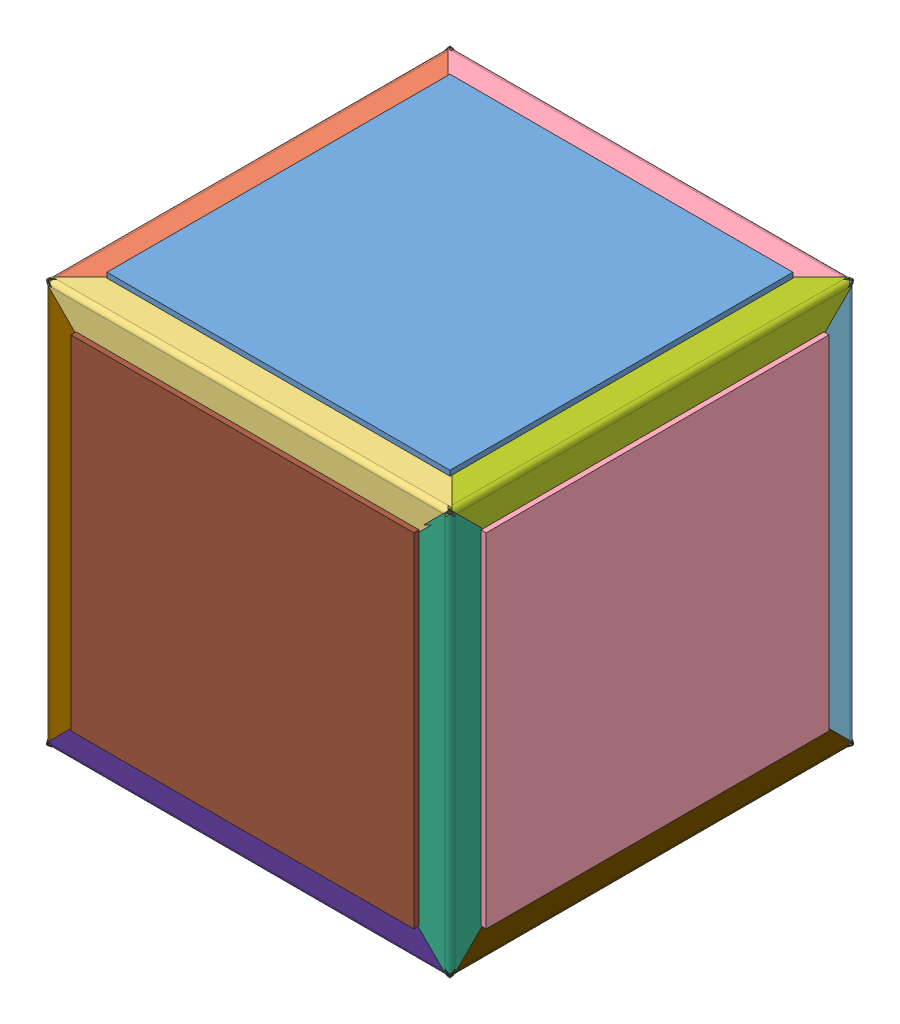
SolidWorks assembly cube_05, configuration cube05. Lengths in mm.
Overall size (127.64 127.64 127.64).
30 component instances, 30 part files, 92 mates.
Components (placement in the parent):
- pr^cube_05-28: pr^cube_05 [cube01] x (-1 0 0) z (0 0 1) size (105.41 1.59 105.41) (virtual)
- dr1^cube_05-55: dr1^cube_05 [cube01] at (-61.6246 62.23 0) x (0 -1 0) z (0 0 1) size (26.01 26.01 124.47) (virtual)
- dr2^cube_05-37: dr2^cube_05 [cube01] at (0 62.23 61.6246) x (0 -1 0) z (1 0 0) size (26.01 26.01 124.47) (virtual)
- dr3^cube_05-33: dr3^cube_05 [cube01] at (0 62.23 -61.6246) x (0 -1 0) z (-1 0 0) size (26.01 26.01 124.47) (virtual)
- br1^cube_05-49: br1^cube_05 [Default] at (0 36.83 -36.83) x (0 0 1) z (-1 0 0) size (50.8 50.8 66.55) (virtual)
- br2^cube_05-61: br2^cube_05 [Default] at (-36.83 36.83 0) size (50.8 50.8 66.55) (virtual)
- br3^cube_05-46: br3^cube_05 [Default] at (0 36.83 36.83) x (0 0 -1) z (1 0 0) size (50.8 50.8 66.55) (virtual)
- pg^cube_05-20: pg^cube_05 [cube01] x (0 -1 0) z (0 0 1) size (105.41 1.59 105.41) (virtual)
- dg1^cube_05-38: dg1^cube_05 [cube01] at (-62.23 0 61.6246) x (1 0 0) z (0 1 0) size (26.01 26.01 124.47) (virtual)
- dg2^cube_05-41: dg2^cube_05 [cube01] at (-62.23 -61.6246 0) size (26.01 26.01 124.47) (virtual)
- dg3^cube_05-34: dg3^cube_05 [cube01] at (-62.23 0 -61.6246) x (1 0 0) z (0 -1 0) size (26.01 26.01 124.47) (virtual)
- bg1^cube_05-47: bg1^cube_05 [Default] at (-36.83 -36.83 0) x (0 1 0) z (0 0 1) size (50.8 50.8 66.55) (virtual)
- bg2^cube_05-44: bg2^cube_05 [Default] at (-36.83 0 36.83) x (0 0 -1) z (0 1 0) size (50.8 50.8 66.55) (virtual)
- bg3^cube_05-40: bg3^cube_05 [Default] at (-36.83 0 -36.83) x (0 0 1) z (0 -1 0) size (50.8 50.8 66.55) (virtual)
- py^cube_05-21: py^cube_05 [cube01] at origin size (105.41 1.59 105.41) (virtual)
- dy1^cube_05-35: dy1^cube_05 [cube01] at (0 -62.23 -61.6246) x (0 1 0) z (1 0 0) size (26.01 26.01 124.47) (virtual)
- dy2^cube_05-39: dy2^cube_05 [cube01] at (0 -62.23 61.6246) x (0 1 0) z (-1 0 0) size (26.01 26.01 124.47) (virtual)
- dy3^cube_05-42: dy3^cube_05 [cube01] at (61.6246 -62.23 0) x (0 1 0) z (0 0 1) size (26.01 26.01 124.47) (virtual)
- by1^cube_05-41: by1^cube_05 [Default] at (0 -36.83 -36.83) x (0 0 1) z (1 0 0) size (50.8 50.8 66.55) (virtual)
- by2^cube_05-45: by2^cube_05 [Default] at (0 -36.83 36.83) x (0 0 -1) z (-1 0 0) size (50.8 50.8 66.55) (virtual)
- by3^cube_05-48: by3^cube_05 [Default] at (36.83 -36.83 0) x (-1 0 0) z (0 0 1) size (50.8 50.8 66.55) (virtual)
- po^cube_05-22: po^cube_05 [cube01] x (0 1 0) z (0 0 1) size (105.41 1.59 105.41) (virtual)
- do1^cube_05-36: do1^cube_05 [cube01] at (62.23 0 -61.6246) x (-1 0 0) z (0 1 0) size (26.01 26.01 124.47) (virtual)
- do2^cube_05-40: do2^cube_05 [cube01] at (62.23 0 61.6246) x (-1 0 0) z (0 -1 0) size (26.01 26.01 124.47) (virtual)
- do3^cube_05-47: do3^cube_05 [cube01] at (62.23 61.6246 0) x (-1 0 0) z (0 0 1) size (26.01 26.01 124.47) (virtual)
- bo1^cube_05-42: bo1^cube_05 [Default] at (36.83 0 -36.83) x (0 0 1) z (0 1 0) size (50.8 50.8 66.55) (virtual)
- bo2^cube_05-46: bo2^cube_05 [Default] at (36.83 0 36.83) x (0 0 -1) z (0 -1 0) size (50.8 50.8 66.55) (virtual)
- bo3^cube_05-62: bo3^cube_05 [Default] at (36.83 36.83 0) x (0 -1 0) z (0 0 1) size (50.8 50.8 66.55) (virtual)
- pc^cube_05-18: pc^cube_05 [cube01] x (-1 0 0) z (0 -1 0) size (105.41 1.59 105.41) (virtual)
- pb^cube_05-21: pb^cube_05 [cube01] x (-1 0 0) z (0 1 0) size (105.41 1.59 105.41) (virtual)
Mates (geometry in assembly coordinates):
- Coincident1: coincident anti-aligned: plane of pr^cube_05-28 through (52.705 62.23 -52.705) normal (0 -1 0); plane of br1^cube_05-49 through (-33.274 62.23 -36.83) normal (0 1 0)
- Coincident2: coincident anti-aligned: plane of pr^cube_05-28 through (52.705 62.23 -52.705) normal (0 -1 0); plane of br2^cube_05-61 through (-36.83 62.23 33.274) normal (0 1 0)
- Coincident3: coincident anti-aligned: plane of pr^cube_05-28 through (52.705 62.23 -52.705) normal (0 -1 0); plane of br3^cube_05-46 through (33.274 62.23 36.83) normal (0 1 0)
- Coincident4: coincident anti-aligned: plane of pr^cube_05-28 through (52.705 62.23 -52.705) normal (0 -1 0); plane of bo3^cube_05-62 through (36.83 62.23 33.274) normal (0 1 0)
- Coincident5: coincident anti-aligned: plane of pr^cube_05-28 through (52.705 62.23 -52.705) normal (0 -1 0); plane of dr3^cube_05-33 through (0 62.23 -123.8546) normal (0 1 0)
- Coincident6: coincident anti-aligned: plane of pr^cube_05-28 through (52.705 62.23 -52.705) normal (0 -1 0); plane of dr1^cube_05-55 through (-123.8546 62.23 0) normal (0 1 0)
- Coincident7: coincident anti-aligned: plane of pr^cube_05-28 through (52.705 62.23 -52.705) normal (0 -1 0); plane of do3^cube_05-47 through (-0.6054 62.23 0) normal (0 1 0)
- Coincident8: coincident anti-aligned: plane of pr^cube_05-28 through (52.705 62.23 -52.705) normal (0 -1 0); plane of dr2^cube_05-37 through (0 62.23 123.8546) normal (0 1 0)
- Coincident34: coincident anti-aligned: plane of pb^cube_05-21 through (52.705 -52.705 -62.23) normal (0 0 1); plane of by1^cube_05-41 through (33.274 -36.83 -62.23) normal (0 0 -1)
- Coincident35: coincident anti-aligned: plane of pb^cube_05-21 through (52.705 -52.705 -62.23) normal (0 0 1); plane of bo1^cube_05-42 through (36.83 33.274 -62.23) normal (0 0 -1)
- Coincident36: coincident anti-aligned: plane of pb^cube_05-21 through (52.705 -52.705 -62.23) normal (0 0 1); plane of br1^cube_05-49 through (-33.274 36.83 -62.23) normal (0 0 -1)
- Coincident37: coincident anti-aligned: plane of pb^cube_05-21 through (52.705 -52.705 -62.23) normal (0 0 1); plane of bg3^cube_05-40 through (-36.83 -33.274 -62.23) normal (0 0 -1)
- Coincident38: coincident anti-aligned: plane of pb^cube_05-21 through (52.705 -52.705 -62.23) normal (0 0 1); plane of dg3^cube_05-34 through (0.6054 0 -62.23) normal (0 0 -1)
- Coincident39: coincident anti-aligned: plane of pb^cube_05-21 through (52.705 -52.705 -62.23) normal (0 0 1); plane of dr3^cube_05-33 through (0 -0.6054 -62.23) normal (0 0 -1)
- Coincident40: coincident anti-aligned: plane of pb^cube_05-21 through (52.705 -52.705 -62.23) normal (0 0 1); plane of do1^cube_05-36 through (-0.6054 0 -62.23) normal (0 0 -1)
- Coincident41: coincident anti-aligned: plane of pb^cube_05-21 through (52.705 -52.705 -62.23) normal (0 0 1); plane of dy1^cube_05-35 through (0 0.6054 -62.23) normal (0 0 -1)
- Coincident42: coincident anti-aligned: plane of pc^cube_05-18 through (52.705 52.705 62.23) normal (0 0 -1); plane of bo2^cube_05-46 through (36.83 -33.274 62.23) normal (0 0 1)
- Coincident43: coincident anti-aligned: plane of pc^cube_05-18 through (52.705 52.705 62.23) normal (0 0 -1); plane of br3^cube_05-46 through (33.274 36.83 62.23) normal (0 0 1)
- Coincident44: coincident anti-aligned: plane of pc^cube_05-18 through (52.705 52.705 62.23) normal (0 0 -1); plane of bg2^cube_05-44 through (-36.83 33.274 62.23) normal (0 0 1)
- Coincident45: coincident anti-aligned: plane of pc^cube_05-18 through (52.705 52.705 62.23) normal (0 0 -1); plane of by2^cube_05-45 through (-33.274 -36.83 62.23) normal (0 0 1)
- Coincident46: coincident anti-aligned: plane of pc^cube_05-18 through (52.705 52.705 62.23) normal (0 0 -1); plane of do2^cube_05-40 through (-0.6054 0 62.23) normal (0 0 1)
- Coincident47: coincident anti-aligned: plane of pc^cube_05-18 through (52.705 52.705 62.23) normal (0 0 -1); plane of dy2^cube_05-39 through (0 0.6054 62.23) normal (0 0 1)
- Coincident48: coincident anti-aligned: plane of pc^cube_05-18 through (52.705 52.705 62.23) normal (0 0 -1); plane of dg1^cube_05-38 through (0.6054 0 62.23) normal (0 0 1)
- Coincident49: coincident anti-aligned: plane of pc^cube_05-18 through (52.705 52.705 62.23) normal (0 0 -1); plane of dr2^cube_05-37 through (0 -0.6054 62.23) normal (0 0 1)
- Coincident50: coincident anti-aligned: plane of pg^cube_05-20 through (-62.23 52.705 -52.705) normal (1 0 0); plane of bg3^cube_05-40 through (-62.23 -33.274 -36.83) normal (-1 0 0)
- Coincident51: coincident anti-aligned: plane of pg^cube_05-20 through (-62.23 52.705 -52.705) normal (1 0 0); plane of bg1^cube_05-47 through (-62.23 -36.83 33.274) normal (-1 0 0)
- Coincident52: coincident anti-aligned: plane of pg^cube_05-20 through (-62.23 52.705 -52.705) normal (1 0 0); plane of bg2^cube_05-44 through (-62.23 33.274 36.83) normal (-1 0 0)
- Coincident53: coincident anti-aligned: plane of pg^cube_05-20 through (-62.23 52.705 -52.705) normal (1 0 0); plane of dr1^cube_05-55 through (-62.23 -0.6054 0) normal (-1 0 0)
- Coincident54: coincident anti-aligned: plane of pg^cube_05-20 through (-62.23 52.705 -52.705) normal (1 0 0); plane of dg3^cube_05-34 through (-62.23 0 -123.8546) normal (-1 0 0)
- Coincident55: coincident anti-aligned: plane of pg^cube_05-20 through (-62.23 52.705 -52.705) normal (1 0 0); plane of dg2^cube_05-41 through (-62.23 -123.8546 0) normal (-1 0 0)
- Coincident56: coincident anti-aligned: plane of pg^cube_05-20 through (-62.23 52.705 -52.705) normal (1 0 0); plane of dg1^cube_05-38 through (-62.23 0 123.8546) normal (-1 0 0)
- Coincident99: coincident anti-aligned: plane of pg^cube_05-20 through (-62.23 52.705 -52.705) normal (1 0 0); plane of br2^cube_05-61 through (-62.23 36.83 33.274) normal (-1 0 0)
- Coincident57: coincident anti-aligned: plane of py^cube_05-21 through (-52.705 -62.23 -52.705) normal (0 1 0); plane of by3^cube_05-48 through (36.83 -62.23 33.274) normal (0 -1 0)
- Coincident58: coincident anti-aligned: plane of py^cube_05-21 through (-52.705 -62.23 -52.705) normal (0 1 0); plane of by2^cube_05-45 through (-33.274 -62.23 36.83) normal (0 -1 0)
- Coincident59: coincident anti-aligned: plane of py^cube_05-21 through (-52.705 -62.23 -52.705) normal (0 1 0); plane of bg1^cube_05-47 through (-36.83 -62.23 33.274) normal (0 -1 0)
- Coincident60: coincident anti-aligned: plane of py^cube_05-21 through (-52.705 -62.23 -52.705) normal (0 1 0); plane of by1^cube_05-41 through (33.274 -62.23 -36.83) normal (0 -1 0)
- Coincident61: coincident anti-aligned: plane of py^cube_05-21 through (-52.705 -62.23 -52.705) normal (0 1 0); plane of dy3^cube_05-42 through (123.8546 -62.23 0) normal (0 -1 0)
- Coincident62: coincident anti-aligned: plane of py^cube_05-21 through (-52.705 -62.23 -52.705) normal (0 1 0); plane of dy2^cube_05-39 through (0 -62.23 123.8546) normal (0 -1 0)
- Coincident63: coincident anti-aligned: plane of py^cube_05-21 through (-52.705 -62.23 -52.705) normal (0 1 0); plane of dg2^cube_05-41 through (0.6054 -62.23 0) normal (0 -1 0)
- Coincident64: coincident anti-aligned: plane of py^cube_05-21 through (-52.705 -62.23 -52.705) normal (0 1 0); plane of dy1^cube_05-35 through (0 -62.23 -123.8546) normal (0 -1 0)
- Coincident65: coincident anti-aligned: plane of po^cube_05-22 through (62.23 -52.705 -52.705) normal (-1 0 0); plane of bo1^cube_05-42 through (62.23 33.274 -36.83) normal (1 0 0)
- Coincident66: coincident anti-aligned: plane of po^cube_05-22 through (62.23 -52.705 -52.705) normal (-1 0 0); plane of by3^cube_05-48 through (62.23 -36.83 33.274) normal (1 0 0)
- Coincident67: coincident anti-aligned: plane of po^cube_05-22 through (62.23 -52.705 -52.705) normal (-1 0 0); plane of bo2^cube_05-46 through (62.23 -33.274 36.83) normal (1 0 0)
- Coincident68: coincident anti-aligned: plane of po^cube_05-22 through (62.23 -52.705 -52.705) normal (-1 0 0); plane of bo3^cube_05-62 through (62.23 36.83 33.274) normal (1 0 0)
- Coincident69: coincident anti-aligned: plane of po^cube_05-22 through (62.23 -52.705 -52.705) normal (-1 0 0); plane of do2^cube_05-40 through (62.23 0 123.8546) normal (1 0 0)
- Coincident70: coincident anti-aligned: plane of po^cube_05-22 through (62.23 -52.705 -52.705) normal (-1 0 0); plane of do3^cube_05-47 through (62.23 123.8546 0) normal (1 0 0)
- Coincident71: coincident anti-aligned: plane of po^cube_05-22 through (62.23 -52.705 -52.705) normal (-1 0 0); plane of do1^cube_05-36 through (62.23 0 -123.8546) normal (1 0 0)
- Coincident72: coincident anti-aligned: plane of po^cube_05-22 through (62.23 -52.705 -52.705) normal (-1 0 0); plane of dy3^cube_05-42 through (62.23 0.6054 0) normal (1 0 0)
- Coincident73: coincident aligned: plane of assembly through (0 0 0) normal (0 0 1); plane of dy3^cube_05-42 through (61.6246 -62.23 0) normal (0 0 1)
- Coincident74: coincident aligned: plane of assembly through (0 0 0) normal (0 0 1); plane of by3^cube_05-48 through (36.83 -36.83 0) normal (0 0 1)
- Coincident75: coincident aligned: plane of assembly through (0 0 0) normal (0 0 1); plane of bo3^cube_05-62 through (36.83 36.83 0) normal (0 0 1)
- Coincident76: coincident aligned: plane of assembly through (0 0 0) normal (0 0 1); plane of do3^cube_05-47 through (62.23 61.6246 0) normal (0 0 1)
- Coincident77: coincident aligned: plane of assembly through (0 0 0) normal (0 0 1); plane of dg2^cube_05-41 through (-62.23 -61.6246 0) normal (0 0 1)
- Coincident78: coincident aligned: plane of assembly through (0 0 0) normal (0 0 1); plane of bg1^cube_05-47 through (-36.83 -36.83 0) normal (0 0 1)
- Coincident79: coincident aligned: plane of assembly through (0 0 0) normal (0 0 1); plane of dr1^cube_05-55 through (-61.6246 62.23 0) normal (0 0 1)
- Coincident80: coincident aligned: plane of assembly through (0 0 0) normal (0 0 1); plane of br2^cube_05-61 through (-36.83 36.83 0) normal (0 0 1)
- Coincident81: coincident aligned: plane of assembly through (0 0 0) normal (0 1 0); plane of bo1^cube_05-42 through (36.83 0 -36.83) normal (0 1 0)
- Coincident82: coincident aligned: plane of assembly through (0 0 0) normal (0 1 0); plane of py^cube_05-21 through (0 0 0) normal (0 1 0)
- Coincident83: coincident aligned: plane of assembly through (0 0 0) normal (0 1 0); plane of do1^cube_05-36 through (62.23 0 -61.6246) normal (0 1 0)
- Coincident84: coincident anti-aligned: plane of assembly through (0 0 0) normal (0 1 0); plane of bg3^cube_05-40 through (-36.83 0 -36.83) normal (0 -1 0)
- Coincident85: coincident anti-aligned: plane of assembly through (0 0 0) normal (0 1 0); plane of dg3^cube_05-34 through (-62.23 0 -61.6246) normal (0 -1 0)
- Coincident86: coincident aligned: plane of assembly through (0 0 0) normal (0 1 0); plane of dg1^cube_05-38 through (-62.23 0 61.6246) normal (0 1 0)
- Coincident87: coincident aligned: plane of assembly through (0 0 0) normal (0 1 0); plane of bg2^cube_05-44 through (-36.83 0 36.83) normal (0 1 0)
- Coincident88: coincident anti-aligned: plane of assembly through (0 0 0) normal (0 1 0); plane of bo2^cube_05-46 through (36.83 0 36.83) normal (0 -1 0)
- Coincident89: coincident anti-aligned: plane of assembly through (0 0 0) normal (0 1 0); plane of do2^cube_05-40 through (62.23 0 61.6246) normal (0 -1 0)
- Coincident90: coincident anti-aligned: plane of assembly through (0 0 0) normal (1 0 0); plane of by2^cube_05-45 through (0 -36.83 36.83) normal (-1 0 0)
- Coincident91: coincident anti-aligned: plane of assembly through (0 0 0) normal (1 0 0); plane of dy2^cube_05-39 through (0 -62.23 61.6246) normal (-1 0 0)
- Coincident92: coincident aligned: plane of assembly through (0 0 0) normal (1 0 0); plane of pg^cube_05-20
- Coincident93: coincident aligned: plane of assembly through (0 0 0) normal (1 0 0); plane of dr2^cube_05-37 through (0 62.23 61.6246) normal (1 0 0)
- Coincident94: coincident aligned: plane of assembly through (0 0 0) normal (1 0 0); plane of br3^cube_05-46 through (0 36.83 36.83) normal (1 0 0)
- Coincident95: coincident anti-aligned: plane of assembly through (0 0 0) normal (1 0 0); plane of dr3^cube_05-33 through (0 62.23 -61.6246) normal (-1 0 0)
- Coincident96: coincident anti-aligned: plane of assembly through (0 0 0) normal (1 0 0); plane of br1^cube_05-49 through (0 36.83 -36.83) normal (-1 0 0)
- Coincident97: coincident aligned: plane of assembly through (0 0 0) normal (1 0 0); plane of by1^cube_05-41 through (0 -36.83 -36.83) normal (1 0 0)
- Coincident98: coincident aligned: plane of assembly through (0 0 0) normal (1 0 0); plane of dy1^cube_05-35 through (0 -62.23 -61.6246) normal (1 0 0)
- Coincident100: coincident anti-aligned: plane of pr^cube_05-28; plane of assembly through (0 0 0) normal (1 0 0)
- Coincident101: coincident aligned: plane of pr^cube_05-28 through (0 0 0) normal (0 0 1); plane of assembly through (0 0 0) normal (0 0 1)
- Coincident102: coincident anti-aligned: plane of pr^cube_05-28; plane of assembly through (0 0 0) normal (0 1 0)
- Coincident106: coincident anti-aligned: plane of pg^cube_05-20; plane of assembly through (0 0 0) normal (0 1 0)
- Coincident107: coincident aligned: plane of pg^cube_05-20; plane of assembly through (0 0 0) normal (1 0 0)
- Coincident108: coincident aligned: plane of pg^cube_05-20 through (0 0 0) normal (0 0 1); plane of assembly through (0 0 0) normal (0 0 1)
- Coincident109: coincident aligned: plane of py^cube_05-21 through (0 0 0) normal (0 0 1); plane of assembly through (0 0 0) normal (0 0 1)
- Coincident110: coincident aligned: plane of py^cube_05-21 through (0 0 0) normal (0 1 0); plane of assembly through (0 0 0) normal (0 1 0)
- Coincident111: coincident aligned: plane of py^cube_05-21 through (0 0 0) normal (1 0 0); plane of assembly through (0 0 0) normal (1 0 0)
- Coincident112: coincident aligned: plane of po^cube_05-22 through (0 0 0) normal (0 0 1); plane of assembly through (0 0 0) normal (0 0 1)
- Coincident113: coincident anti-aligned: plane of po^cube_05-22; plane of assembly through (0 0 0) normal (1 0 0)
- Coincident114: coincident aligned: plane of po^cube_05-22; plane of assembly through (0 0 0) normal (0 1 0)
- Coincident115: coincident anti-aligned: plane of pc^cube_05-18 through (0 0 0) normal (0 -1 0); plane of assembly through (0 0 0) normal (0 1 0)
- Coincident116: coincident anti-aligned: plane of pc^cube_05-18; plane of assembly through (0 0 0) normal (0 0 1)
- Coincident117: coincident anti-aligned: plane of pc^cube_05-18; plane of assembly through (0 0 0) normal (1 0 0)
- Coincident118: coincident aligned: plane of pb^cube_05-21 through (0 0 0) normal (0 1 0); plane of assembly through (0 0 0) normal (0 1 0)
- Coincident119: coincident aligned: plane of pb^cube_05-21; plane of assembly through (0 0 0) normal (0 0 1)
- Coincident120: coincident anti-aligned: line of pb^cube_05-21 through (0.8731 -0.8731 0) axis (0 0 -1); plane of assembly through (0 0 0) normal (1 0 0)
